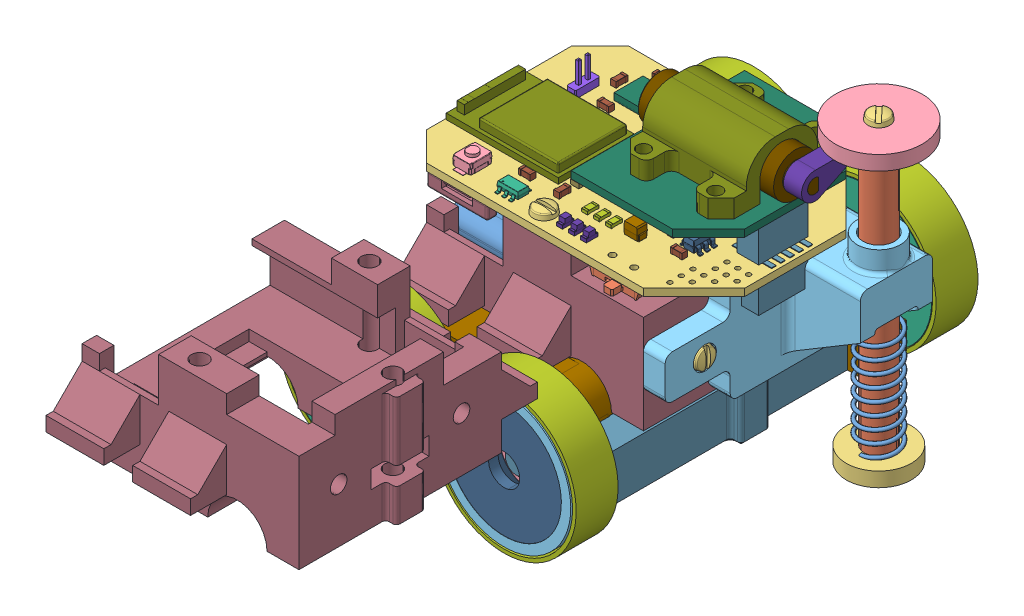
SolidWorks assembly AstroAnt_small_magnet, configuration Default. Lengths in mm.
Overall size (52.48 43.35 103.22).
156 component instances, 41 part files, 86 mates.
Components (placement in the parent):
- LiPo_360mAh-1: LiPo_360mAh [Default] at (6.0099 4.9998 47.0256) size (26.5 4.2 23.5)
- 92120A150_Brass Heat-Set Inserts for Plastic-1: 92120A150_Brass Heat-Set Inserts for Plastic [92120A150] at (19.9543 12.4998 45.7029) size (2.56 3.33 2.56)
- 92120A150_Brass Heat-Set Inserts for Plastic-2: 92120A150_Brass Heat-Set Inserts for Plastic [92120A150] at (4.9543 12.4998 33.9529) size (2.56 3.33 2.56)
- 92120A150_Brass Heat-Set Inserts for Plastic-3: 92120A150_Brass Heat-Set Inserts for Plastic [92120A150] at (4.9543 12.4998 57.4529) size (2.56 3.33 2.56)
- 91460A005_METRIC CHEESE HEAD SLOTTED MACHINE SCREW-8: 91460A005_METRIC CHEESE HEAD SLOTTED MACHINE SCREW [91460A005] at (4.9543 14.9998 57.4529) x (1 0 0) z (0 1 0) size (3 3 7.1)
- 91460A005_METRIC CHEESE HEAD SLOTTED MACHINE SCREW-9: 91460A005_METRIC CHEESE HEAD SLOTTED MACHINE SCREW [91460A005] at (4.9543 14.9998 33.9529) x (1 0 0) z (0 1 0) size (3 3 7.1)
- 91460A005_METRIC CHEESE HEAD SLOTTED MACHINE SCREW-10: 91460A005_METRIC CHEESE HEAD SLOTTED MACHINE SCREW [91460A005] at (19.9543 14.9998 45.7029) x (1 0 0) z (0 1 0) size (3 3 7.1)
- 92120A150_Brass Heat-Set Inserts for Plastic-4: 92120A150_Brass Heat-Set Inserts for Plastic [92120A150] at (4.9543 -0.6002 57.4529) x (-0.616962 0 -0.786993) z (0.786993 0 -0.616962) size (2.56 3.33 2.56)
- 92120A150_Brass Heat-Set Inserts for Plastic-5: 92120A150_Brass Heat-Set Inserts for Plastic [92120A150] at (4.9543 -0.6002 33.9529) x (-0.616962 0 -0.786993) z (0.786993 0 -0.616962) size (2.56 3.33 2.56)
- mainboard_v1.step-1: mainboard_v1.step [Default] at (-103.0457 13.9998 235.7029) x (0 0 -1) z (0 1 0) size (29.41 41 10.8)
  - B3U-1000P.step-1: B3U-1000P.step [Default] at (178.95 -97.38 1.05) x (1 0 0) z (0 -1 0) size (4 1.75 2.5)
    - COMPOUND.step-1: COMPOUND.step [Default] at origin size (4 1.75 2.5)
  - 20021321-00014C1LF.step-1: 20021321-00014C1LF.step [Default] at (190 -115.5 1.05) size (9.35 5.45 4.85)
    - COMPOUND-0.step-1: COMPOUND-0.step [Default] at origin size (9.35 5.45 4.85)
  - MP6513GJ-Z.step-1: MP6513GJ-Z.step [Default] at (201.21 -120 1.05) x (-1 0 0) z (0 0 1) size (2.8 2.9 1)
    - COMPOUND-1.step-1: COMPOUND-1.step [Default] at origin size (2.8 2.9 1)
  - MP6513GJ-Z.step-2: MP6513GJ-Z.step [Default] at (178.51 -103.46 1.05) size (2.8 2.9 1)
    - COMPOUND-1.step-1: COMPOUND-1.step [Default] at origin size (2.8 2.9 1)
  - R_0603_1608Metric.step-1: R_0603_1608Metric.step [Default] at (195.55 -104.38 -0.05) x (1 0 0) z (0 0 -1) size (1.6 0.8 0.45)
    - SOLID.step-1: SOLID.step [Default] at origin size (1.6 0.8 0.45)
  - R_0603_1608Metric.step-2: R_0603_1608Metric.step [Default] at (192.6 -99.86 -0.05) x (0 1 0) z (0 0 -1) size (1.6 0.8 0.45)
    - SOLID.step-1: SOLID.step [Default] at origin size (1.6 0.8 0.45)
  - PinHeader_2x01_P1.27mm_Vertical.step-1: PinHeader_2x01_P1.27mm_Vertical.step [Default] at (194.96 -96.07 1.05) size (3.4 1.27 6.3)
    - SOLID-2.step-1: SOLID-2.step [Default] at origin size (3.4 1.27 6.3)
  - TAJP106K010RNJ.step-1: TAJP106K010RNJ.step [Default] at (196.22 -98.14 -0.05) x (-1 0 0) z (0 0 -1) size (2.05 1.4 1.7)
    - COMPOUND-3.step-1: COMPOUND-3.step [Default] at origin size (2.05 1.4 1.7)
  - TAJP106K010RNJ.step-2: TAJP106K010RNJ.step [Default] at (181.68 -117.23 1.05) x (0 1 0) z (0 0 1) size (2.05 1.4 1.7)
    - COMPOUND-3.step-1: COMPOUND-3.step [Default] at origin size (2.05 1.4 1.7)
  - SOT-23-5.step-1: SOT-23-5.step [Default] at (195.38 -122.78 1.05) x (0 1 0) z (0 0 1) size (2.8 2.9 1.55)
    - SOLID-4.step-1: SOLID-4.step [Default] at origin size (2.8 2.9 1.55)
  - C_0603_1608Metric.step-1: C_0603_1608Metric.step [Default] at (192.91 -122.55 1.05) x (0 -1 0) z (0 0 1) size (1.6 0.8 0.8)
    - SOLID-5.step-1: SOLID-5.step [Default] at origin size (1.6 0.8 0.8)
  - C_0603_1608Metric.step-2: C_0603_1608Metric.step [Default] at (193.57 -119.76 1.05) size (1.6 0.8 0.8)
    - SOLID-5.step-1: SOLID-5.step [Default] at origin size (1.6 0.8 0.8)
  - ECS-.327-12.5-12-TR.step-1: ECS-.327-12.5-12-TR.step [Default] at (184.31 -107.18 1.05) size (2 1.2 0.7)
    - COMPOUND-6.step-1: COMPOUND-6.step [Default] at origin size (2 1.2 0.7)
  - C_0603_1608Metric.step-3: C_0603_1608Metric.step [Default] at (197.67 -113.69 1.05) size (1.6 0.8 0.8)
    - SOLID-5.step-1: SOLID-5.step [Default] at origin size (1.6 0.8 0.8)
  - C_0603_1608Metric.step-4: C_0603_1608Metric.step [Default] at (197.64 -107.18 1.05) size (1.6 0.8 0.8)
    - SOLID-5.step-1: SOLID-5.step [Default] at origin size (1.6 0.8 0.8)
  - C_0603_1608Metric.step-5: C_0603_1608Metric.step [Default] at (190.96 -108.09 1.05) x (0 1 0) z (0 0 1) size (1.6 0.8 0.8)
    - SOLID-5.step-1: SOLID-5.step [Default] at origin size (1.6 0.8 0.8)
  - 1734592-6.step-1: 1734592-6.step [Default] at (203.79 -118 -1.05) x (0 -1 0) z (1 0 0) size (8.43 2.05 5.11)
    - SOLID-7.step-1: SOLID-7.step [Default] at origin size (8.43 2.05 5.11)
  - 1734592-6.step-2: 1734592-6.step [Default] at (176.19 -98 -1.05) x (0 1 0) z (-1 0 0) size (8.43 2.05 5.11)
    - SOLID-7.step-1: SOLID-7.step [Default] at origin size (8.43 2.05 5.11)
  - 20021321-00010C4LF.step-1: 20021321-00010C4LF.step [Default] at (190 -127.85 -0.05) x (1 0 0) z (0 0 -1) size (6.81 5.45 4.85)
    - COMPOUND-8.step-1: COMPOUND-8.step [Default] at origin size (6.81 5.45 4.85)
  - 20021321-00010C4LF.step-2: 20021321-00010C4LF.step [Default] at (190 -127.85 1.05) size (6.81 5.45 4.85)
    - COMPOUND-8.step-1: COMPOUND-8.step [Default] at origin size (6.81 5.45 4.85)
  - C_0603_1608Metric.step-6: C_0603_1608Metric.step [Default] at (181.31 -102.6 1.05) x (0 -1 0) z (0 0 1) size (1.6 0.8 0.8)
    - SOLID-5.step-1: SOLID-5.step [Default] at origin size (1.6 0.8 0.8)
  - C_0603_1608Metric.step-7: C_0603_1608Metric.step [Default] at (198.25 -119.14 1.05) x (0 -1 0) z (0 0 1) size (1.6 0.8 0.8)
    - SOLID-5.step-1: SOLID-5.step [Default] at origin size (1.6 0.8 0.8)
  - MPU6050.step-1: MPU6050.step [Default] at (198.43 -101.5 1.05) x (0 1 0) z (1 0 0) size (4 0.95 4)
    - COMPOUND-9.step-1: COMPOUND-9.step [Default] at origin size (4 0.95 4)
  - C_0603_1608Metric.step-8: C_0603_1608Metric.step [Default] at (194.9 -99.89 1.05) x (0 -1 0) z (0 0 1) size (1.6 0.8 0.8)
    - SOLID-5.step-1: SOLID-5.step [Default] at origin size (1.6 0.8 0.8)
  - C_0603_1608Metric.step-9: C_0603_1608Metric.step [Default] at (201.98 -100.38 1.05) x (0 -1 0) z (0 0 1) size (1.6 0.8 0.8)
    - SOLID-5.step-1: SOLID-5.step [Default] at origin size (1.6 0.8 0.8)
  - C_0603_1608Metric.step-10: C_0603_1608Metric.step [Default] at (201.98 -103.78 1.05) x (0 1 0) z (0 0 1) size (1.6 0.8 0.8)
    - SOLID-5.step-1: SOLID-5.step [Default] at origin size (1.6 0.8 0.8)
  - C_0603_1608Metric.step-11: C_0603_1608Metric.step [Default] at (198.81 -97.82 1.05) size (1.6 0.8 0.8)
    - SOLID-5.step-1: SOLID-5.step [Default] at origin size (1.6 0.8 0.8)
  - SOT-23-5.step-2: SOT-23-5.step [Default] at (184.86 -122.77 1.05) x (0 1 0) z (0 0 1) size (2.8 2.9 1.55)
    - SOLID-4.step-1: SOLID-4.step [Default] at origin size (2.8 2.9 1.55)
  - SOT-23-5.step-3: SOT-23-5.step [Default] at (197.58 -110.46 1.05) x (0 1 0) z (0 0 1) size (2.8 2.9 1.55)
    - SOLID-4.step-1: SOLID-4.step [Default] at origin size (2.8 2.9 1.55)
  - MDBT50Q-1MV2.step-1: MDBT50Q-1MV2.step [Default] at (187.3136 -98.605 1.0754) x (-1 0 0) z (0 1 0) size (10.5 2.06 15.5)
    - SOLID-10.step-1: SOLID-10.step [Default] at origin size (10.5 2.06 15.5)
  - C_0603_1608Metric.step-12: C_0603_1608Metric.step [Default] at (189.44 -108.09 1.05) x (0 1 0) z (0 0 1) size (1.6 0.8 0.8)
    - SOLID-5.step-1: SOLID-5.step [Default] at origin size (1.6 0.8 0.8)
  - C_0603_1608Metric.step-13: C_0603_1608Metric.step [Default] at (181.57 -107.18 1.05) x (-1 0 0) z (0 0 1) size (1.6 0.8 0.8)
    - SOLID-5.step-1: SOLID-5.step [Default] at origin size (1.6 0.8 0.8)
  - C_0603_1608Metric.step-14: C_0603_1608Metric.step [Default] at (186.97 -107.18 1.05) size (1.6 0.8 0.8)
    - SOLID-5.step-1: SOLID-5.step [Default] at origin size (1.6 0.8 0.8)
  - C_0603_1608Metric.step-15: C_0603_1608Metric.step [Default] at (184.77 -119.75 1.05) x (-1 0 0) z (0 0 1) size (1.6 0.8 0.8)
    - SOLID-5.step-1: SOLID-5.step [Default] at origin size (1.6 0.8 0.8)
  - C_0603_1608Metric.step-16: C_0603_1608Metric.step [Default] at (182.37 -122.54 1.05) x (0 -1 0) z (0 0 1) size (1.6 0.8 0.8)
    - SOLID-5.step-1: SOLID-5.step [Default] at origin size (1.6 0.8 0.8)
  - LED_0603_1608Metric.step-1: LED_0603_1608Metric.step [Default] at (178.19 -111.01 1.05) size (1.6 0.8 1.1)
    - SOLID-11.step-1: SOLID-11.step [Default] at origin size (1.6 0.8 1.1)
  - LED_0603_1608Metric.step-2: LED_0603_1608Metric.step [Default] at (178.19 -112.66 1.05) size (1.6 0.8 1.1)
    - SOLID-11.step-1: SOLID-11.step [Default] at origin size (1.6 0.8 1.1)
  - LED_0603_1608Metric.step-3: LED_0603_1608Metric.step [Default] at (178.19 -114.31 1.05) size (1.6 0.8 1.1)
    - SOLID-11.step-1: SOLID-11.step [Default] at origin size (1.6 0.8 1.1)
  - LED_0603_1608Metric.step-4: LED_0603_1608Metric.step [Default] at (202.34 -112.21 1.05) x (0 1 0) z (0 0 1) size (1.6 0.8 1.1)
    - SOLID-11.step-1: SOLID-11.step [Default] at origin size (1.6 0.8 1.1)
  - 473460001.step-1: 473460001.step [Default] at (201.68 -99.72 -1.25) x (0 -1 0) z (1 0 0) size (7.98 2.94 5.43)
    - COMPOUND-12.step-1: COMPOUND-12.step [Default] at origin size (7.98 2.94 5.43)
  - L_0603_1608Metric.step-1: L_0603_1608Metric.step [Default] at (192.48 -108.09 1.05) x (0 1 0) z (0 0 1) size (1.6 0.8 0.8)
    - SOLID-13.step-1: SOLID-13.step [Default] at origin size (1.6 0.8 0.8)
  - R_0603_1608Metric.step-3: R_0603_1608Metric.step [Default] at (185.18 -111.31 1.05) x (-1 0 0) z (0 0 1) size (1.6 0.8 0.45)
    - SOLID.step-1: SOLID.step [Default] at origin size (1.6 0.8 0.45)
  - R_0603_1608Metric.step-4: R_0603_1608Metric.step [Default] at (185.18 -109.77 1.05) size (1.6 0.8 0.45)
    - SOLID.step-1: SOLID.step [Default] at origin size (1.6 0.8 0.45)
  - R_0603_1608Metric.step-5: R_0603_1608Metric.step [Default] at (181.62 -111.01 1.05) size (1.6 0.8 0.45)
    - SOLID.step-1: SOLID.step [Default] at origin size (1.6 0.8 0.45)
  - R_0603_1608Metric.step-6: R_0603_1608Metric.step [Default] at (181.62 -112.66 1.05) size (1.6 0.8 0.45)
    - SOLID.step-1: SOLID.step [Default] at origin size (1.6 0.8 0.45)
  - R_0603_1608Metric.step-7: R_0603_1608Metric.step [Default] at (181.62 -114.31 1.05) x (-1 0 0) z (0 0 1) size (1.6 0.8 0.45)
    - SOLID.step-1: SOLID.step [Default] at origin size (1.6 0.8 0.45)
  - R_0603_1608Metric.step-8: R_0603_1608Metric.step [Default] at (194.84 -108.1 1.05) x (0 1 0) z (0 0 1) size (1.6 0.8 0.45)
    - SOLID.step-1: SOLID.step [Default] at origin size (1.6 0.8 0.45)
  - R_0603_1608Metric.step-9: R_0603_1608Metric.step [Default] at (200.69 -112.2325 1.05) x (0 1 0) z (0 0 1) size (1.6 0.8 0.45)
    - SOLID.step-1: SOLID.step [Default] at origin size (1.6 0.8 0.45)
  - R_0603_1608Metric.step-10: R_0603_1608Metric.step [Default] at (196.22 -101.51 -0.05) x (-1 0 0) z (0 0 -1) size (1.6 0.8 0.45)
    - SOLID.step-1: SOLID.step [Default] at origin size (1.6 0.8 0.45)
  - R_0603_1608Metric.step-11: R_0603_1608Metric.step [Default] at (196.22 -99.9725 -0.05) x (-1 0 0) z (0 0 -1) size (1.6 0.8 0.45)
    - SOLID.step-1: SOLID.step [Default] at origin size (1.6 0.8 0.45)
  - SW_SPDT_PCM12.step-1: SW_SPDT_PCM12.step [Default] at (178.18 -119.37 -0.05) x (0 1 0) z (0 0 -1) size (7.7 5 2)
    - SOLID-14.step-1: SOLID-14.step [Default] at origin size (7.7 5 2)
  - COMPOUND-15.step-1: COMPOUND-15.step [Default] at origin size (28 41 1)
- ball_bearing_5x11x4mm-1: ball_bearing_5x11x4mm [Default] at (-65.9801 -4.7758 21.2029) x (0.999925 -0.012245 0) z (0 0 1) size (8 8 2.5)
- wheel_holder_non_motor-1: wheel_holder_non_motor [Default] at (-90.7699 -0.8362 17.9029) size (18.5 18.5 5.8)
- wheel_holder_non_motor-2: wheel_holder_non_motor [Default] at (1.3792 -86.6559 73.5029) x (0.185441 0.982655 0) z (0 0 -1) size (18.5 18.5 5.8)
- ball_bearing_5x11x4mm-2: ball_bearing_5x11x4mm [Default] at (-9.788 -57.5376 70.2029) x (0.373101 0.927791 0) z (0 0 -1) size (8 8 2.5)
- wheel_motor-1: wheel_motor [Default] at (44.5289 -0.8963 17.9029) size (18.8 18.8 5.8)
- wheel_motor-2: wheel_motor [Default] at (-4.9746 26.526 73.5029) x (-0.038296 0.999266 0) z (0 0 -1) size (18.8 18.8 5.8)
- tire-1: tire [Default] at (58.6593 -4.042 17.9029) size (20 20 5.8)
- tire-2: tire [Default] at (37.6493 -4.042 17.9029) size (20 20 5.8)
- tire-3: tire [Default] at (58.6593 -4.042 67.7029) size (20 20 5.8)
- tire-4: tire [Default] at (37.6493 -4.042 67.7029) size (20 20 5.8)
- PA2-50_with_gearbox-3: PA2-50_with_gearbox [Default] at (45.51 -3.6027 60.1029) x (-1 0 0) z (0 0 1) size (30.92 12.52 38.5)
  - PA2-50-1: PA2-50 [Default] at (26.117 -19.7771 -19.1) x (0 0 1) z (0.954024 0.299729 0) size (29.1 8 8)
  - gearbox-1: gearbox [Default] at origin size (29.9 11.5 13.6)
- PA2-50_with_gearbox-4: PA2-50_with_gearbox [Default] at (-35.6268 -3.6027 31.3029) x (1 0 0) z (0 0 -1) size (30.92 12.52 38.5)
  - PA2-50-1: PA2-50 [Default] at (26.117 -19.7771 -19.1) x (0 0 1) z (0.954024 0.299729 0) size (29.1 8 8)
  - gearbox-1: gearbox [Default] at origin size (29.9 11.5 13.6)
- RA22CS-N-1: RA22CS-N [Default] at (15.4466 -2.6002 19.5154) x (1 0 0) z (0 -1 0) size (15.88 3.17 15.88)
- RA22CS-N-2: RA22CS-N [Default] at (-5.5634 -2.6002 19.5154) x (1 0 0) z (0 -1 0) size (15.88 3.17 15.88)
- RA22CS-N-3: RA22CS-N [Default] at (-5.5634 -2.6002 71.8904) x (-0.968047 -0.250767 0) z (0.250767 -0.968047 0) size (15.88 3.17 15.88)
- RA22CS-N-4: RA22CS-N [Default] at (15.4466 -2.6002 71.8904) x (-0.968047 -0.250767 0) z (0.250767 -0.968047 0) size (15.88 3.17 15.88)
- TPiS_1084-1: TPiS_1084 [Default] at (-17.7438 -7.4002 31.4743) size (9.3 10.3 10.11)
- IR_TEMP_module-1: IR_TEMP_module [Default] at (15.0895 3.8498 50.7532) x (0 0 -1) z (0 1 0) size (10 20 1.85)
- robobody-1: robobody [Default] at (-9.0457 6.9406 -0.9986) size (31.5 16.1 38)
- 92120A150_Brass Heat-Set Inserts for Plastic-6: 92120A150_Brass Heat-Set Inserts for Plastic [92120A150] at (19.9543 -0.6002 45.7029) x (-0.616962 0 -0.786993) z (0.786993 0 -0.616962) size (2.56 3.33 2.56)
- motor_holder_2-1: motor_holder_2 [Default] at (52.4112 -9.4002 -5.2676) size (31.5 8.8 52.2)
- 92120A150_Brass Heat-Set Inserts for Plastic-7: 92120A150_Brass Heat-Set Inserts for Plastic [92120A150] at (19.4543 5.3998 54.2029) x (0 1 0) z (0 0 1) size (2.56 3.33 2.56)
- 92120A150_Brass Heat-Set Inserts for Plastic-8: 92120A150_Brass Heat-Set Inserts for Plastic [92120A150] at (19.4543 5.3998 37.2029) x (0 1 0) z (0 0 1) size (2.56 3.33 2.56)
- knocking_knob-2: knocking_knob [Default] at (-34.3202 21.0998 1.0679) size (19 1 24)
- knock_motor_holder-1: knock_motor_holder [Default] at (-0.3495 22.1998 0.3235) size (14.34 7 16.88)
- knock_wheel-1: knock_wheel [Default] at (28.1543 -28.5709 73.2155) x (1 0 0) z (0 1 0) size (2.5 8.21 3.71)
- TGPP06-D-136-1: TGPP06-D-136 [Default] at (9.0543 25.0998 45.7013) x (0 -1 0) z (1 0 0) size (6 6 21.6)
- spring-1: spring [Default] at (30.9214 -10.0489 37.1029) size (6.35 16 5.5)
- knockknock_knob-1: knockknock_knob [Default] at (30.9214 -10.0489 37.1029) x (0.999972 0 -0.007535) z (0.007535 0 0.999972) size (4 37 4)
- 92120A150_Brass Heat-Set Inserts for Plastic-9: 92120A150_Brass Heat-Set Inserts for Plastic [92120A150] at (30.9214 -8.5489 37.1029) x (-0.616962 0 -0.786993) z (0.786993 0 -0.616962) size (2.56 3.33 2.56)
- 91460A005_METRIC CHEESE HEAD SLOTTED MACHINE SCREW-11: 91460A005_METRIC CHEESE HEAD SLOTTED MACHINE SCREW [91460A005] at (30.9214 -12.0489 37.1029) x (-0.226988 0 -0.973897) z (0 -1 0) size (3 3 7.1)
- 92120A150_Brass Heat-Set Inserts for Plastic-10: 92120A150_Brass Heat-Set Inserts for Plastic [92120A150] at (30.9214 25.4511 37.1029) x (0.427311 0 -0.904105) z (0.904105 0 0.427311) size (2.56 3.33 2.56)
- 91460A005_METRIC CHEESE HEAD SLOTTED MACHINE SCREW-12: 91460A005_METRIC CHEESE HEAD SLOTTED MACHINE SCREW [91460A005] at (30.9214 28.9511 37.1029) x (-0.681379 0 -0.731931) z (0 1 0) size (3 3 7.1)
- knocking_head-3: knocking_head [Default] at (-47.1305 -12.0489 -34.3498) size (9 2 9)
- kncoking_head_2-1: kncoking_head_2 [Default] at (3.2885 26.9511 24.2097) size (12 2 12)
- knocking_holder-1: knocking_holder [Default] at (20.9543 37.9038 -8.5349) size (13 17 27)
- 91460A005_METRIC CHEESE HEAD SLOTTED MACHINE SCREW-13: 91460A005_METRIC CHEESE HEAD SLOTTED MACHINE SCREW [91460A005] at (23.4543 5.3998 54.2029) x (0 -1 0) z (1 0 0) size (3 3 7.1)
- 91460A005_METRIC CHEESE HEAD SLOTTED MACHINE SCREW-14: 91460A005_METRIC CHEESE HEAD SLOTTED MACHINE SCREW [91460A005] at (23.4543 5.3998 37.2029) x (0 -1 0) z (1 0 0) size (3 3 7.1)
- robobody-2: robobody [Default] at (-0.3034 22.882 55.4177) size (31.5 16.1 38)
Mates (geometry in assembly coordinates):
- Concentric63: concentric anti-aligned: cylinder of ball_bearing_5x11x4mm-1 through (-5.5634 -2.6002 23.7029) axis (0 0 -1) radius 4; cylinder of wheel_holder_non_motor-1 through (-5.5634 -2.6002 17.9029) axis (0 0 1) radius 4
- Coincident105: coincident aligned: plane of ball_bearing_5x11x4mm-1 through (-5.5634 -2.6002 23.7029) normal (0 0 1); plane of wheel_holder_non_motor-1 through (-5.5634 -2.6002 23.7029) normal (0 0 1)
- Coincident107: coincident aligned: plane of wheel_holder_non_motor-2 through (15.4466 -2.6002 67.7029) normal (0 0 -1); plane of ball_bearing_5x11x4mm-2 through (15.4466 -2.6002 67.7029) normal (0 0 -1)
- Concentric83: concentric anti-aligned: cylinder of wheel_motor-1 through (15.4466 -2.6002 23.7029) axis (0 0 -1) radius 9.4; cylinder of tire-1 through (15.4466 -2.6002 17.9029) axis (0 0 1) radius 9.5
- Coincident123: coincident aligned: plane of wheel_motor-1 through (15.4466 -2.6002 17.9029) normal (0 0 -1); plane of tire-1 through (15.4466 -2.6002 17.9029) normal (0 0 -1)
- Concentric84: concentric anti-aligned: cylinder of wheel_holder_non_motor-1 through (-5.5634 -2.6002 23.7029) axis (0 0 -1) radius 9.25; cylinder of tire-2 through (-5.5634 -2.6002 17.9029) axis (0 0 1) radius 9.5
- Coincident124: coincident aligned: plane of wheel_holder_non_motor-1 through (-5.5634 -2.6002 17.9029) normal (0 0 -1); plane of tire-2 through (-5.5634 -2.6002 17.9029) normal (0 0 -1)
- Coincident125: coincident aligned: plane of wheel_motor-2 through (-5.5634 -2.6002 73.5029) normal (0 0 1); plane of tire-4 through (-5.5634 -2.6002 73.5029) normal (0 0 1)
- Concentric85: concentric aligned: cylinder of wheel_motor-2 through (-5.5634 -2.6002 67.7029) axis (0 0 1) radius 9.4; cylinder of tire-4 through (-5.5634 -2.6002 67.7029) axis (0 0 1) radius 9.5
- Coincident126: coincident aligned: plane of wheel_holder_non_motor-2 through (15.4466 -2.6002 73.5029) normal (0 0 1); plane of tire-3 through (15.4466 -2.6002 73.5029) normal (0 0 1)
- Concentric86: concentric aligned: cylinder of wheel_holder_non_motor-2 through (15.4466 -2.6002 67.7029) axis (0 0 1) radius 9.25; cylinder of tire-3 through (15.4466 -2.6002 67.7029) axis (0 0 1) radius 9.5
- Concentric100: concentric anti-aligned: cylinder of wheel_holder_non_motor-2 through (15.4466 -2.6002 73.5029) axis (0 0 -1) radius 4; cylinder of ball_bearing_5x11x4mm-2 through (15.4466 -2.6002 66.2029) axis (0 0 1) radius 2
- Coincident138: coincident aligned: plane of wheel_holder_non_motor-2 through (15.4466 -2.6002 67.7029) normal (0 0 -1); plane of ball_bearing_5x11x4mm-2 through (15.4466 -2.6002 67.7029) normal (0 0 -1)
- Concentric110: concentric anti-aligned: cylinder of wheel_motor-2 through (-5.5634 -2.6002 67.7029) axis (0 0 1) radius 1.4; cylinder of PA2-50_with_gearbox-3/gearbox-1 through (-5.5634 -2.6002 71.7029) axis (0 0 -1) radius 1.45
- Concentric111: concentric aligned: cylinder of tire-1 through (15.4466 -2.6002 23.7029) axis (0 0 -1) radius 10; cylinder of tire-3 through (15.4466 -2.6002 73.5029) axis (0 0 -1) radius 10
- Concentric112: concentric aligned: cylinder of tire-2 through (-5.5634 -2.6002 23.7029) axis (0 0 -1) radius 10; cylinder of tire-4 through (-5.5634 -2.6002 73.5029) axis (0 0 -1) radius 10
- Coincident144: coincident aligned: plane of PA2-50_with_gearbox-3/gearbox-1 through (16.4366 -9.1002 65.7029) normal (0 -1 0); plane of PA2-50_with_gearbox-4/gearbox-1 through (-6.5534 -9.1002 25.7029) normal (0 -1 0)
- Coincident145: coincident aligned: plane of wheel_holder_non_motor-1 through (-5.5634 -2.6002 17.9029) normal (0 0 -1); plane of wheel_motor-1 through (15.4466 -2.6002 17.9029) normal (0 0 -1)
- Coincident146: coincident aligned: plane of wheel_holder_non_motor-2 through (15.4466 -2.6002 73.5029) normal (0 0 1); plane of wheel_motor-2 through (-5.5634 -2.6002 73.5029) normal (0 0 1)
- Coincident149: coincident anti-aligned: plane of wheel_motor-1 through (15.4466 -2.6002 21.1029) normal (0 0 -1); plane of RA22CS-N-1 through (15.4466 -2.6002 21.1029) normal (0 0 1)
- Concentric113: concentric aligned: cylinder of wheel_motor-1 through (15.4466 -2.6002 23.7029) axis (0 0 -1) radius 1.4; cylinder of RA22CS-N-1 through (15.4466 -2.6002 19.5154) axis (0 0 -1) radius 2.159
- Concentric114: concentric aligned: cylinder of wheel_holder_non_motor-1 through (-5.5634 -2.6002 21.1029) axis (0 0 -1) radius 7.95; cylinder of RA22CS-N-2 through (-5.5634 -2.6002 19.5154) axis (0 0 -1) radius 2.159
- Coincident150: coincident anti-aligned: plane of wheel_holder_non_motor-1 through (-5.5634 -2.6002 21.1029) normal (0 0 -1); plane of RA22CS-N-2 through (-5.5634 -2.6002 21.1029) normal (0 0 1)
- Concentric115: concentric aligned: cylinder of wheel_motor-2 through (-5.5634 -2.6002 70.3029) axis (0 0 1) radius 7.95; cylinder of RA22CS-N-3 through (-5.5634 -2.6002 70.3029) axis (0 0 1) radius 7.9375
- Coincident151: coincident anti-aligned: plane of wheel_motor-2 through (-5.5634 -2.6002 70.3029) normal (0 0 1); plane of RA22CS-N-3 through (-5.5634 -2.6002 70.3029) normal (0 0 -1)
- Concentric116: concentric aligned: cylinder of wheel_holder_non_motor-2 through (15.4466 -2.6002 70.3029) axis (0 0 1) radius 7.95; cylinder of RA22CS-N-4 through (15.4466 -2.6002 70.3029) axis (0 0 1) radius 7.9375
- Coincident152: coincident anti-aligned: plane of wheel_holder_non_motor-2 through (15.4466 -2.6002 70.3029) normal (0 0 1); plane of RA22CS-N-4 through (15.4466 -2.6002 70.3029) normal (0 0 -1)
- Concentric118: concentric anti-aligned: cylinder of TPiS_1084-1 through (2.2416 -0.7002 46.8203) axis (0 -1 0) radius 0.225; cylinder of IR_TEMP_module-1 through (2.2414 3.8498 46.8208) axis (0 1 0) radius 0.3
- Concentric119: concentric anti-aligned: cylinder of TPiS_1084-1 through (3.8219 -0.7002 43.0052) axis (0 -1 0) radius 0.225; cylinder of IR_TEMP_module-1 through (3.8219 3.8498 43.0052) axis (0 1 0) radius 0.3
- Coincident153: coincident aligned: plane of mainboard_v1.step-1/COMPOUND-15.step-1 through (20.9543 13.9998 59.7029) normal (0 0 1); plane of robobody-1 through (20.9543 13.9998 59.7029) normal (0 0 1)
- Coincident154: coincident: line of mainboard_v1.step-1/COMPOUND-15.step-1 through (-9.0457 13.9998 59.7029) axis (0 1 0); plane of robobody-1 through (-9.0457 6.9406 -0.9986) normal (-1 0 0)
- Parallel1: parallel: line of IR_TEMP_module-1 through (15.0895 3.8498 50.7532) axis (-1 0 0); plane of robobody-1 through (-8.0457 3.9998 55.2029) normal (0 0 -1)
- Concentric121: concentric aligned: cylinder of 92120A150_Brass Heat-Set Inserts for Plastic-4 through (4.9543 0.8998 57.4529) axis (0 1 0) radius 1.075; cylinder of robobody-1 through (4.9543 -2.1591 57.4529) axis (0 1 0) radius 1.15
- Concentric122: concentric aligned: cylinder of 92120A150_Brass Heat-Set Inserts for Plastic-5 through (4.9543 0.8998 33.9529) axis (0 1 0) radius 1.075; cylinder of robobody-1 through (4.9543 -2.1591 33.9529) axis (0 1 0) radius 1.15
- Concentric123: concentric aligned: cylinder of robobody-1 through (19.9543 -2.1591 45.7029) axis (0 1 0) radius 1.15; cylinder of 92120A150_Brass Heat-Set Inserts for Plastic-6 through (19.9543 0.8998 45.7029) axis (0 1 0) radius 1.075
- Coincident164: coincident anti-aligned: plane of PA2-50_with_gearbox-4/gearbox-1 through (12.2966 -5.4002 30.3029) normal (0 -1 0); plane of motor_holder_2-1 through (-9.0457 -5.4002 31.5029) normal (0 1 0)
- Coincident167: coincident aligned: plane of robobody-1 through (20.9543 6.9406 -0.9986) normal (1 0 0); plane of motor_holder_2-1 through (20.9543 -2.4002 61.1029) normal (1 0 0)
- Coincident168: coincident anti-aligned: plane of TPiS_1084-1 through (4.9393 -7.4002 45.7029) normal (0 -1 0); plane of motor_holder_2-1 through (4.9393 -7.4002 45.7029) normal (0 1 0)
- Coincident169: coincident anti-aligned: plane of TPiS_1084-1 through (4.9393 -7.4002 45.7029) normal (0 -1 0); plane of motor_holder_2-1 through (4.9393 -7.4002 45.7029) normal (0 1 0)
- Coincident170: coincident anti-aligned: plane of TPiS_1084-1 through (4.9393 -7.4002 45.7029) normal (0 -1 0); plane of motor_holder_2-1 through (4.9393 -7.4002 45.7029) normal (0 1 0)
- Concentric124: concentric anti-aligned: cylinder of PA2-50_with_gearbox-3/PA2-50-1 through (12.4366 -2.1002 57.2029) axis (0 0 -1) radius 4; cylinder of robobody-1 through (12.4366 -2.1002 32.5029) axis (0 0 1) radius 4.1
- Concentric125: concentric anti-aligned: cylinder of PA2-50_with_gearbox-4/PA2-50-1 through (-2.5534 -2.1002 34.2029) axis (0 0 1) radius 4; cylinder of robobody-1 through (-2.5534 -2.1002 58.9029) axis (0 0 -1) radius 4.1
- Coincident174: coincident anti-aligned: plane of PA2-50_with_gearbox-4/gearbox-1 through (-2.5534 -2.1002 31.7029) normal (0 0 1); plane of robobody-1 through (20.9543 13.9998 31.7029) normal (0 0 -1)
- Coincident175: coincident anti-aligned: plane of PA2-50_with_gearbox-3/gearbox-1 through (12.4366 -2.1002 59.7029) normal (0 0 -1); plane of robobody-1 through (20.9543 13.9998 59.7029) normal (0 0 1)
- Coincident176: coincident anti-aligned: plane of mainboard_v1.step-1/COMPOUND-15.step-1 through (6.7692 13.9998 45.7029) normal (0 -1 0); plane of robobody-1 through (20.9543 13.9998 59.7029) normal (0 1 0)
- Concentric126: concentric anti-aligned: cylinder of robobody-1 through (14.5016 5.3998 54.2029) axis (1 0 0) radius 1.15; cylinder of 92120A150_Brass Heat-Set Inserts for Plastic-7 through (17.9543 5.3998 54.2029) axis (-1 0 0) radius 1.075
- Concentric127: concentric anti-aligned: cylinder of robobody-1 through (14.5016 5.3998 37.2029) axis (1 0 0) radius 1.15; cylinder of 92120A150_Brass Heat-Set Inserts for Plastic-8 through (17.9543 5.3998 37.2029) axis (-1 0 0) radius 1.075
- Coincident177: coincident aligned: plane of robobody-1 through (20.9543 6.9406 -0.9986) normal (1 0 0); plane of 92120A150_Brass Heat-Set Inserts for Plastic-8 through (20.9543 4.5998 37.2029) normal (1 0 0)
- Coincident178: coincident aligned: plane of robobody-1 through (20.9543 6.9406 -0.9986) normal (1 0 0); plane of 92120A150_Brass Heat-Set Inserts for Plastic-7 through (20.9543 4.5998 54.2029) normal (1 0 0)
- Distance1: distance = 2 mm anti-aligned: plane of wheel_motor-2 through (-5.5634 -2.6002 67.7029) normal (0 0 -1); plane of PA2-50_with_gearbox-3/gearbox-1 through (45.51 -3.6027 65.7029) normal (0 0 1)
- Distance2: distance = 2 mm anti-aligned: plane of wheel_motor-1 through (15.4466 -2.6002 23.7029) normal (0 0 1); plane of PA2-50_with_gearbox-4/gearbox-1 through (-35.6268 -3.6027 25.7029) normal (0 0 -1)
- Concentric128: concentric anti-aligned: cylinder of PA2-50_with_gearbox-4/gearbox-1 through (15.4466 -2.6002 19.7029) axis (0 0 1) radius 1.45; cylinder of RA22CS-N-1 through (15.4466 -2.6002 19.5154) axis (0 0 -1) radius 2.159
- Coincident183: coincident anti-aligned: line of mainboard_v1.step-1/COMPOUND-15.step-1 through (27.9543 13.9998 38.7029) axis (0 1 0); line of knocking_knob-2 through (27.9543 22.0998 38.7029) axis (0 -1 0)
- Distance3: distance = 1.2 mm anti-aligned: plane of knocking_knob-2 through (-34.3202 21.0998 1.0679) normal (0 -1 0); plane of mainboard_v1.step-1/20021321-00010C4LF.step-2/COMPOUND-8.step-1 through (24.8043 19.8998 45.7029) normal (0 1 0)
- Coincident185: coincident aligned: plane of mainboard_v1.step-1/COMPOUND-15.step-1 through (27.9543 13.9998 38.7029) normal (1 0 0); plane of knocking_knob-2 through (27.9543 22.0998 38.7029) normal (1 0 0)
- Concentric129: concentric aligned: cylinder of knocking_knob-2 through (13.9543 21.0998 38.7029) axis (0 1 0) radius 0.9; cylinder of knock_motor_holder-1 through (13.9543 22.1998 38.7029) axis (0 1 0) radius 0.9
- Concentric130: concentric aligned: cylinder of knock_motor_holder-1 through (26.1243 25.0998 45.7013) axis (-1 0 0) radius 3.05; cylinder of TGPP06-D-136-1 through (27.9543 25.0998 45.7013) axis (-1 0 0) radius 3
- Coincident187: coincident aligned: plane of knocking_knob-2 through (27.9543 22.0998 38.7029) normal (1 0 0); plane of TGPP06-D-136-1 through (27.9543 25.0998 45.7013) normal (1 0 0)
- Tangent1: tangent anti-aligned: plane of knocking_knob-2 through (-34.3202 22.0998 1.0679) normal (0 1 0); cylinder of TGPP06-D-136-1 through (27.9543 25.0998 45.7013) axis (-1 0 0) radius 3
- Coincident191: coincident aligned: plane of knock_wheel-1 through (30.6543 25.0998 42.5751) normal (1 0 0); plane of TGPP06-D-136-1 through (30.6543 25.0998 45.7013) normal (1 0 0)
- Coincident199: coincident aligned: plane of knockknock_knob-1 through (30.9214 -10.0489 37.1029) normal (0 -1 0); plane of 92120A150_Brass Heat-Set Inserts for Plastic-9 through (31.415 -10.0489 37.7325) normal (0 -1 0)
- Concentric136: concentric anti-aligned: cylinder of knockknock_knob-1 through (30.9214 26.9511 37.1029) axis (0 -1 0) radius 2; cylinder of 92120A150_Brass Heat-Set Inserts for Plastic-9 through (30.9214 -7.0489 37.1029) axis (0 1 0) radius 1.075
- Concentric137: concentric aligned: circle of spring-1; circle of knockknock_knob-1
- Concentric138: concentric anti-aligned: cylinder of knock_wheel-1 through (28.1543 25.0998 45.7013) axis (1 0 0) radius 0.99; cylinder of TGPP06-D-136-1 through (27.9543 25.0998 45.7013) axis (-1 0 0) radius 3
- Parallel11: parallel aligned: plane of knocking_knob-2 through (-34.3202 22.0998 1.0679) normal (0 1 0); plane of knock_wheel-1 through (20.9137 26.9511 45.5738) normal (0 1 0)
- Coincident202: coincident anti-aligned: circle of spring-1; plane of knockknock_knob-1 through (30.9214 -10.0489 37.1029) normal (0 -1 0)
- Distance6: distance = 5.4 mm: cylinder of knockknock_knob-1 through (30.9214 26.9511 37.1029) axis (0 -1 0) radius 2; plane of robobody-1 through (20.9543 13.9998 31.7029) normal (0 0 -1)
- Distance7: distance = 2 mm anti-aligned: plane of 91460A005_METRIC CHEESE HEAD SLOTTED MACHINE SCREW-11 through (30.9214 -12.0489 37.1029) normal (0 1 0); plane of knockknock_knob-1 through (30.9214 -10.0489 37.1029) normal (0 -1 0)
- Concentric139: concentric aligned: circle of knockknock_knob-1; circle of 91460A005_METRIC CHEESE HEAD SLOTTED MACHINE SCREW-11
- Concentric140: concentric anti-aligned: cylinder of knockknock_knob-1 through (30.9214 26.9511 37.1029) axis (0 -1 0) radius 2; cylinder of 92120A150_Brass Heat-Set Inserts for Plastic-10 through (30.9214 26.9511 37.1029) axis (0 1 0) radius 1.075
- Coincident208: coincident aligned: plane of knockknock_knob-1 through (30.9214 26.9511 37.1029) normal (0 1 0); plane of 92120A150_Brass Heat-Set Inserts for Plastic-10 through (30.4621 26.9511 38.0748) normal (0 1 0)
- Concentric141: concentric anti-aligned: circle of knockknock_knob-1; circle of 91460A005_METRIC CHEESE HEAD SLOTTED MACHINE SCREW-12
- Distance8: distance = 2 mm anti-aligned: plane of 91460A005_METRIC CHEESE HEAD SLOTTED MACHINE SCREW-12 through (30.9214 28.9511 37.1029) normal (0 -1 0); plane of knockknock_knob-1 through (30.9214 26.9511 37.1029) normal (0 1 0)
- Coincident212: coincident anti-aligned: plane of knockknock_knob-1 through (30.9214 -10.0489 37.1029) normal (0 -1 0); plane of knocking_head-3 through (30.9214 -10.0489 37.1029) normal (0 1 0)
- Concentric143: concentric anti-aligned: cylinder of knockknock_knob-1 through (30.9214 26.9511 37.1029) axis (0 -1 0) radius 1.15; cylinder of knocking_head-3 through (30.9214 -12.0489 37.1029) axis (0 1 0) radius 0.9
- Coincident215: coincident anti-aligned: plane of knockknock_knob-1 through (30.9214 26.9511 37.1029) normal (0 1 0); plane of kncoking_head_2-1 through (30.9214 26.9511 37.1029) normal (0 -1 0)
- Concentric144: concentric anti-aligned: cylinder of knockknock_knob-1 through (30.9214 26.9511 37.1029) axis (0 -1 0) radius 1.15; cylinder of kncoking_head_2-1 through (30.9214 26.9511 37.1029) axis (0 1 0) radius 0.9
- Coincident216: coincident anti-aligned: plane of robobody-1 through (20.9543 6.9406 -0.9986) normal (1 0 0); plane of knocking_holder-1 through (20.9543 37.9038 -8.5349) normal (-1 0 0)
- Coincident217: coincident aligned: plane of robobody-1 through (20.9543 13.9998 59.7029) normal (0 0 1); plane of knocking_holder-1 through (23.9543 8.3998 59.7029) normal (0 0 1)
- Concentric145: concentric aligned: cylinder of robobody-1 through (14.5016 5.3998 54.2029) axis (1 0 0) radius 1.15; cylinder of knocking_holder-1 through (20.9543 5.3998 54.2029) axis (1 0 0) radius 0.9
- Coincident219: coincident anti-aligned: plane of knocking_holder-1 through (23.4543 5.3998 54.2029) normal (1 0 0); plane of 91460A005_METRIC CHEESE HEAD SLOTTED MACHINE SCREW-13 through (23.4543 5.3998 54.2029) normal (-1 0 0)
- Concentric146: concentric anti-aligned: circle of knocking_holder-1; circle of 91460A005_METRIC CHEESE HEAD SLOTTED MACHINE SCREW-13
- Concentric147: concentric aligned: circle of knocking_holder-1; circle of 91460A005_METRIC CHEESE HEAD SLOTTED MACHINE SCREW-14
- Coincident220: coincident anti-aligned: plane of knocking_holder-1 through (23.4543 5.3998 37.2029) normal (1 0 0); plane of 91460A005_METRIC CHEESE HEAD SLOTTED MACHINE SCREW-14 through (23.4543 5.3998 37.2029) normal (-1 0 0)
- Distance9: distance = 0.25 mm anti-aligned: plane of LiPo_360mAh-1 through (15.7543 9.1998 57.4529) normal (0 0 1); plane of robobody-1 through (42.4929 9.9998 57.7029) normal (0 0 -1)
- Coincident222: coincident anti-aligned: plane of LiPo_360mAh-1 through (17.7543 4.9998 47.0256) normal (1 0 0); plane of robobody-1 through (17.7543 3.9998 36.2029) normal (-1 0 0)
